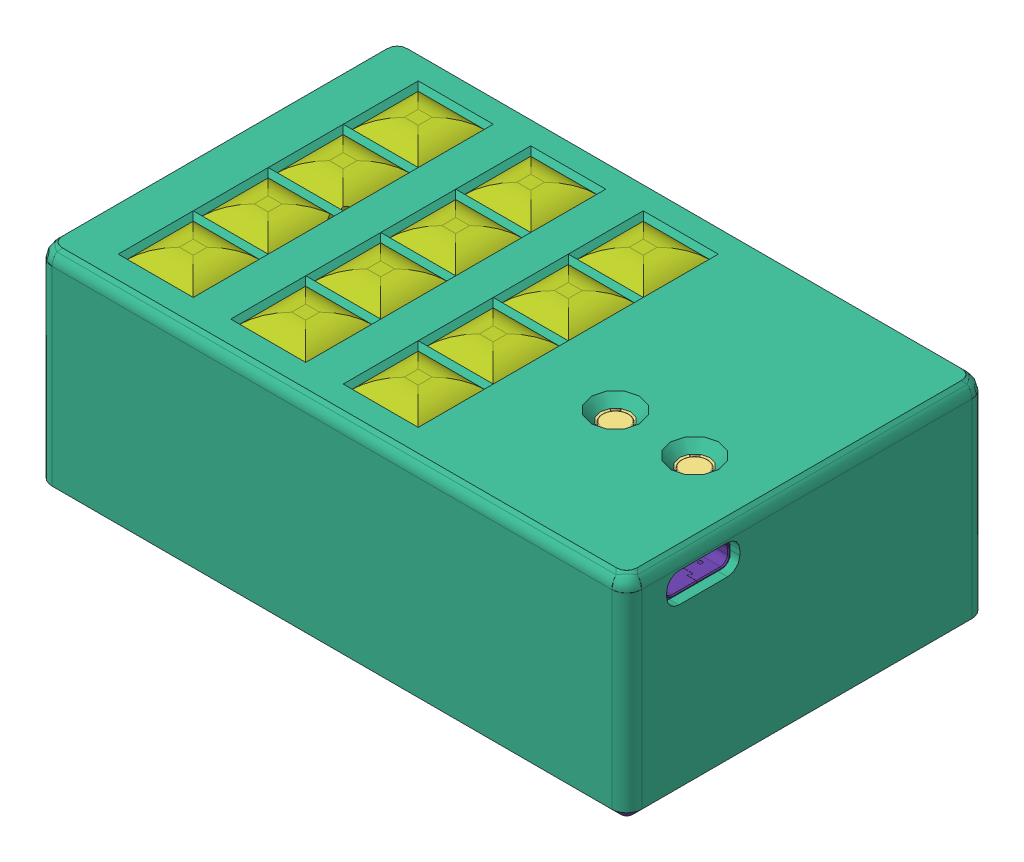
SolidWorks assembly case_mood, configuration Default. Lengths in mm.
Overall size (78.6 29.2 48).
109 component instances, 27 part files, 18 mates.
Components (placement in the parent):
- mood-mood.step-1: mood-mood.step [Default] at (29.4 28.6305 75.6923) x (-1 0 0) z (0 1 0) size (76.01 40 14.44)
  - Board_Geoms_e038.step-1: Board_Geoms_e038.step [Default] at origin size (75 40 1.6)
    - Pcb_e038.step-1: Pcb_e038.step [Default] at (-147.1 99.5 0) size (75 40 1.6)
  - Step_Models_e038.step-1: Step_Models_e038.step [Default] at origin size (71.91 38.55 14.44)
    - Top_e038.step-1: Top_e038.step [Default] at origin size (71.91 38.55 7.8)
      - IC2_DRL0006A_ASM_d850ca76bd89.step-1: IC2_DRL0006A_ASM_d850ca76bd89.step [Default] at (-11.65 2.75 0) size (1.6 1.6 0.6)
        - FRAME-DRL0006A.step-1: FRAME-DRL0006A.step [Default] x (0 1 0) z (1 0 0) size (1.2 0.13 1.6)
          - SOLID.step-1: SOLID.step [Default] at origin size (0.2 0.13 0.3)
          - SOLID001.step-1: SOLID001.step [Default] at origin size (0.2 0.13 0.3)
          - SOLID002.step-1: SOLID002.step [Default] at origin size (0.2 0.13 0.3)
          - SOLID003.step-1: SOLID003.step [Default] at origin size (0.2 0.13 0.3)
          - SOLID004.step-1: SOLID004.step [Default] at origin size (0.2 0.13 0.3)
          - SOLID005.step-1: SOLID005.step [Default] at origin size (0.2 0.13 0.3)
        - BODY-SOT.step-1: BODY-SOT.step [Default] at (0 0 0.025) x (0 1 0) z (1 0 0) size (1.6 0.58 1.2)
      - IC6_ASSEMBLY_ace8437915b6.step-1: IC6_ASSEMBLY_ace8437915b6.step [Default] at (-21.4 7.5 0) size (2.1 2 0.6)
        - Body.step-1: Body.step [Default] at origin size (2 2 0.55)
        - ThermalPin.step-1: ThermalPin.step [Default] at (-0.3875 -0.8375 0) size (0.78 1.68 0.07)
        - PinsArrayLR.step-1: PinsArrayLR.step [Default] at origin size (2.1 1.24 0.07)
      - R52_R_0402_1005Metric_0573c14c30cb.step-1: R52_R_0402_1005Metric_0573c14c30cb.step [Default] at (15.2 -25 0) x (-1 0 0) z (0 0 1) size (1 0.5 0.35)
      - R52_R_0402_1005Metric_0573c14c30cb.step-2: R52_R_0402_1005Metric_0573c14c30cb.step [Default] at (30.2 6.8 0) x (-1 0 0) z (0 0 1) size (1 0.5 0.35)
      - R52_R_0402_1005Metric_0573c14c30cb.step-3: R52_R_0402_1005Metric_0573c14c30cb.step [Default] at (15.2 -6.8 0) x (-1 0 0) z (0 0 1) size (1 0.5 0.35)
      - D4_LED_RGB_5050_6_5aed774da48c.step-1: D4_LED_RGB_5050_6_5aed774da48c.step [Default] at (25 5 0) size (5.4 5 1.6)
      - R52_R_0402_1005Metric_0573c14c30cb.step-4: R52_R_0402_1005Metric_0573c14c30cb.step [Default] at (0.2 -23.2 0) x (-1 0 0) z (0 0 1) size (1 0.5 0.35)
      - IC1_ESP32-C3-WROOM-02-H4_28caeafe01dd.step-1: IC1_ESP32-C3-WROOM-02-H4_28caeafe01dd.step [Default] at (-26.65 -20 0.4) x (-1 0 0) z (0 0 1) size (18 20 3.2)
      - R2_R_0603_1608Metric_003f984474a4.step-1: R2_R_0603_1608Metric_003f984474a4.step [Default] at (-8.65 0 0) x (0 -1 0) z (0 0 1) size (1.6 0.8 0.45)
      - C5_C_0805_2012Metric_cb7698a6af10.step-1: C5_C_0805_2012Metric_cb7698a6af10.step [Default] at (-11.65 0.25 0) size (2 1.25 1.25)
      - R52_R_0402_1005Metric_0573c14c30cb.step-5: R52_R_0402_1005Metric_0573c14c30cb.step [Default] at (30.4 -13.2 0) x (-1 0 0) z (0 0 1) size (1 0.5 0.35)
      - D4_LED_RGB_5050_6_5aed774da48c.step-2: D4_LED_RGB_5050_6_5aed774da48c.step [Default] at (-5 5 0) size (5.4 5 1.6)
      - R52_R_0402_1005Metric_0573c14c30cb.step-6: R52_R_0402_1005Metric_0573c14c30cb.step [Default] at (15.2 -5 0) x (-1 0 0) z (0 0 1) size (1 0.5 0.35)
      - D4_LED_RGB_5050_6_5aed774da48c.step-3: D4_LED_RGB_5050_6_5aed774da48c.step [Default] at (-5 -15 0) size (5.4 5 1.6)
      - R52_R_0402_1005Metric_0573c14c30cb.step-7: R52_R_0402_1005Metric_0573c14c30cb.step [Default] at (15.2 3.2 0) x (-1 0 0) z (0 0 1) size (1 0.5 0.35)
      - D4_LED_RGB_5050_6_5aed774da48c.step-4: D4_LED_RGB_5050_6_5aed774da48c.step [Default] at (10 -15 0) size (5.4 5 1.6)
      - R2_R_0603_1608Metric_003f984474a4.step-2: R2_R_0603_1608Metric_003f984474a4.step [Default] at (-38.1 -17.8 0) x (0 1 0) z (0 0 1) size (1.6 0.8 0.45)
      - R52_R_0402_1005Metric_0573c14c30cb.step-8: R52_R_0402_1005Metric_0573c14c30cb.step [Default] at (30.4 -3.2 0) x (-1 0 0) z (0 0 1) size (1 0.5 0.35)
      - J2_12401610E42A_931c68c1d1c5[2].step-1: J2_12401610E42A_931c68c1d1c5[2].step [Default] at (-41 3.8 1.5) x (-1 0 0) z (0 0 1) size (10.51 9.21 4.22)
      - R2_R_0603_1608Metric_003f984474a4.step-3: R2_R_0603_1608Metric_003f984474a4.step [Default] at (-19 1.6 0) x (0 -1 0) z (0 0 1) size (1.6 0.8 0.45)
      - D4_LED_RGB_5050_6_5aed774da48c.step-5: D4_LED_RGB_5050_6_5aed774da48c.step [Default] at (10 -25 0) size (5.4 5 1.6)
      - R52_R_0402_1005Metric_0573c14c30cb.step-9: R52_R_0402_1005Metric_0573c14c30cb.step [Default] at (30.4 -16.8 0) x (-1 0 0) z (0 0 1) size (1 0.5 0.35)
      - R2_R_0603_1608Metric_003f984474a4.step-4: R2_R_0603_1608Metric_003f984474a4.step [Default] at (-4.65 0.75 0) x (-1 0 0) z (0 0 1) size (1.6 0.8 0.45)
      - R52_R_0402_1005Metric_0573c14c30cb.step-10: R52_R_0402_1005Metric_0573c14c30cb.step [Default] at (15.2025 5 0) x (-1 0 0) z (0 0 1) size (1 0.5 0.35)
      - R2_R_0603_1608Metric_003f984474a4.step-5: R2_R_0603_1608Metric_003f984474a4.step [Default] at (4.5875 -7.2687 0) size (1.6 0.8 0.45)
      - D2_LED_0805_2012Metric_59915ddbd9d1.step-1: D2_LED_0805_2012Metric_59915ddbd9d1.step [Default] at (-21 1.6 0) x (0 -1 0) z (0 0 1) size (2 1.25 1.1)
      - D4_LED_RGB_5050_6_5aed774da48c.step-6: D4_LED_RGB_5050_6_5aed774da48c.step [Default] at (-5 -25 0) size (5.4 5 1.6)
      - R52_R_0402_1005Metric_0573c14c30cb.step-11: R52_R_0402_1005Metric_0573c14c30cb.step [Default] at (0.2 -25 0) x (-1 0 0) z (0 0 1) size (1 0.5 0.35)
      - R52_R_0402_1005Metric_0573c14c30cb.step-12: R52_R_0402_1005Metric_0573c14c30cb.step [Default] at (0.2 3.2 0) x (-1 0 0) z (0 0 1) size (1 0.5 0.35)
      - R52_R_0402_1005Metric_0573c14c30cb.step-13: R52_R_0402_1005Metric_0573c14c30cb.step [Default] at (15.2 -23.2 0) x (-1 0 0) z (0 0 1) size (1 0.5 0.35)
      - R2_R_0603_1608Metric_003f984474a4.step-6: R2_R_0603_1608Metric_003f984474a4.step [Default] at (-14.3 -20.8 0) x (-1 0 0) z (0 0 1) size (1.6 0.8 0.45)
      - R52_R_0402_1005Metric_0573c14c30cb.step-14: R52_R_0402_1005Metric_0573c14c30cb.step [Default] at (30.4 -25 0) x (-1 0 0) z (0 0 1) size (1 0.5 0.35)
      - C11_C_0603_1608Metric_8816bd15a2e3.step-1: C11_C_0603_1608Metric_8816bd15a2e3.step [Default] at (-18.65 7.75 0) x (0 1 0) z (0 0 1) size (1.6 0.8 0.8)
      - D4_LED_RGB_5050_6_5aed774da48c.step-7: D4_LED_RGB_5050_6_5aed774da48c.step [Default] at (25 -25 0) size (5.4 5 1.6)
      - R52_R_0402_1005Metric_0573c14c30cb.step-15: R52_R_0402_1005Metric_0573c14c30cb.step [Default] at (0.2 -3.2 0) x (-1 0 0) z (0 0 1) size (1 0.5 0.35)
      - R2_R_0603_1608Metric_003f984474a4.step-7: R2_R_0603_1608Metric_003f984474a4.step [Default] at (-27.2 0.8 0) x (0 1 0) z (0 0 1) size (1.6 0.8 0.45)
      - C11_C_0603_1608Metric_8816bd15a2e3.step-2: C11_C_0603_1608Metric_8816bd15a2e3.step [Default] at (-11.65 -4 0) size (1.6 0.8 0.8)
      - R52_R_0402_1005Metric_0573c14c30cb.step-16: R52_R_0402_1005Metric_0573c14c30cb.step [Default] at (30.4 -15 0) x (-1 0 0) z (0 0 1) size (1 0.5 0.35)
      - R52_R_0402_1005Metric_0573c14c30cb.step-17: R52_R_0402_1005Metric_0573c14c30cb.step [Default] at (0.2 5 0) x (-1 0 0) z (0 0 1) size (1 0.5 0.35)
      - C11_C_0603_1608Metric_8816bd15a2e3.step-3: C11_C_0603_1608Metric_8816bd15a2e3.step [Default] at (-7.15 0 0) x (0 1 0) z (0 0 1) size (1.6 0.8 0.8)
      - R52_R_0402_1005Metric_0573c14c30cb.step-18: R52_R_0402_1005Metric_0573c14c30cb.step [Default] at (0.2 -6.8 0) x (-1 0 0) z (0 0 1) size (1 0.5 0.35)
      - R2_R_0603_1608Metric_003f984474a4.step-8: R2_R_0603_1608Metric_003f984474a4.step [Default] at (-14.3 -14.4 0) x (-1 0 0) z (0 0 1) size (1.6 0.8 0.45)
      - D4_LED_RGB_5050_6_5aed774da48c.step-8: D4_LED_RGB_5050_6_5aed774da48c.step [Default] at (25 -15 0) size (5.4 5 1.6)
      - R52_R_0402_1005Metric_0573c14c30cb.step-19: R52_R_0402_1005Metric_0573c14c30cb.step [Default] at (30.2 5 0) x (-1 0 0) z (0 0 1) size (1 0.5 0.35)
      - R2_R_0603_1608Metric_003f984474a4.step-9: R2_R_0603_1608Metric_003f984474a4.step [Default] at (4.5875 -17.2063 0) size (1.6 0.8 0.45)
      - D4_LED_RGB_5050_6_5aed774da48c.step-9: D4_LED_RGB_5050_6_5aed774da48c.step [Default] at (10 -5 0) size (5.4 5 1.6)
      - R2_R_0603_1608Metric_003f984474a4.step-10: R2_R_0603_1608Metric_003f984474a4.step [Default] at (-14.3 -17.6 0) size (1.6 0.8 0.45)
      - R2_R_0603_1608Metric_003f984474a4.step-11: R2_R_0603_1608Metric_003f984474a4.step [Default] at (-25.2 1.6 0) x (0 -1 0) z (0 0 1) size (1.6 0.8 0.45)
      - R52_R_0402_1005Metric_0573c14c30cb.step-20: R52_R_0402_1005Metric_0573c14c30cb.step [Default] at (30.4 -6.8 0) x (-1 0 0) z (0 0 1) size (1 0.5 0.35)
      - R2_R_0603_1608Metric_003f984474a4.step-12: R2_R_0603_1608Metric_003f984474a4.step [Default] at (-38.1 -14.4 0) x (0 1 0) z (0 0 1) size (1.6 0.8 0.45)
      - R52_R_0402_1005Metric_0573c14c30cb.step-21: R52_R_0402_1005Metric_0573c14c30cb.step [Default] at (15.2 6.8 0) x (-1 0 0) z (0 0 1) size (1 0.5 0.35)
      - R52_R_0402_1005Metric_0573c14c30cb.step-22: R52_R_0402_1005Metric_0573c14c30cb.step [Default] at (15.2025 -3.2 0) x (-1 0 0) z (0 0 1) size (1 0.5 0.35)
      - R52_R_0402_1005Metric_0573c14c30cb.step-23: R52_R_0402_1005Metric_0573c14c30cb.step [Default] at (30.2 3.2 0) x (-1 0 0) z (0 0 1) size (1 0.5 0.35)
      - Q2_SOT_23_dd72da5cd8d7.step-1: Q2_SOT_23_dd72da5cd8d7.step [Default] at (4.55 -24.1188 0) x (0 1 0) z (0 0 1) size (2.5 3 1.2)
      - R52_R_0402_1005Metric_0573c14c30cb.step-24: R52_R_0402_1005Metric_0573c14c30cb.step [Default] at (30.4 -26.8 0) x (-1 0 0) z (0 0 1) size (1 0.5 0.35)
      - C11_C_0603_1608Metric_8816bd15a2e3.step-4: C11_C_0603_1608Metric_8816bd15a2e3.step [Default] at (-11.7 -19.9 0) x (0 1 0) z (0 0 1) size (1.6 0.8 0.8)
      - R2_R_0603_1608Metric_003f984474a4.step-13: R2_R_0603_1608Metric_003f984474a4.step [Default] at (-38.1 -21.3 0) x (0 1 0) z (0 0 1) size (1.6 0.8 0.45)
      - C5_C_0805_2012Metric_cb7698a6af10.step-2: C5_C_0805_2012Metric_cb7698a6af10.step [Default] at (-10.65 7 0) size (2 1.25 1.25)
      - SW2_SW_PUSH_6mm_h4.3mm_68b5b15dd36c.step-1: SW2_SW_PUSH_6mm_h4.3mm_68b5b15dd36c.step [Default] at (-18 -7.4 0) x (-1 0 0) z (0 0 1) size (7.17 6 7.8)
      - R52_R_0402_1005Metric_0573c14c30cb.step-25: R52_R_0402_1005Metric_0573c14c30cb.step [Default] at (15.2 -13.2 0) x (-1 0 0) z (0 0 1) size (1 0.5 0.35)
      - R52_R_0402_1005Metric_0573c14c30cb.step-26: R52_R_0402_1005Metric_0573c14c30cb.step [Default] at (15.2 -26.8 0) x (-1 0 0) z (0 0 1) size (1 0.5 0.35)
      - R2_R_0603_1608Metric_003f984474a4.step-14: R2_R_0603_1608Metric_003f984474a4.step [Default] at (-21.4 5.25 0) size (1.6 0.8 0.45)
      - C11_C_0603_1608Metric_8816bd15a2e3.step-5: C11_C_0603_1608Metric_8816bd15a2e3.step [Default] at (-14.3 -22.5 0) size (1.6 0.8 0.8)
      - D4_LED_RGB_5050_6_5aed774da48c.step-10: D4_LED_RGB_5050_6_5aed774da48c.step [Default] at (25 -5 0) size (5.4 5 1.6)
      - SW2_SW_PUSH_6mm_h4.3mm_68b5b15dd36c.step-2: SW2_SW_PUSH_6mm_h4.3mm_68b5b15dd36c.step [Default] at (-34.85 -2.9 0) size (7.17 6 7.8)
      - R52_R_0402_1005Metric_0573c14c30cb.step-27: R52_R_0402_1005Metric_0573c14c30cb.step [Default] at (0.2 -5 0) x (-1 0 0) z (0 0 1) size (1 0.5 0.35)
      - R2_R_0603_1608Metric_003f984474a4.step-15: R2_R_0603_1608Metric_003f984474a4.step [Default] at (-29 0.8 0) x (0 1 0) z (0 0 1) size (1.6 0.8 0.45)
      - C5_C_0805_2012Metric_cb7698a6af10.step-3: C5_C_0805_2012Metric_cb7698a6af10.step [Default] at (-11.65 -2 0) size (2 1.25 1.25)
      - D4_LED_RGB_5050_6_5aed774da48c.step-11: D4_LED_RGB_5050_6_5aed774da48c.step [Default] at (10 5 0) size (5.4 5 1.6)
      - R52_R_0402_1005Metric_0573c14c30cb.step-28: R52_R_0402_1005Metric_0573c14c30cb.step [Default] at (15.2 -16.8 0) x (-1 0 0) z (0 0 1) size (1 0.5 0.35)
      - L1_L_Wuerth_MAPI_4020_5ef69c3bf382.step-1: L1_L_Wuerth_MAPI_4020_5ef69c3bf382.step [Default] at (-15.65 1.75 0) x (0 1 0) z (0 0 1) size (3 4 2)
      - R2_R_0603_1608Metric_003f984474a4.step-16: R2_R_0603_1608Metric_003f984474a4.step [Default] at (-14.3 -19.2 0) x (-1 0 0) z (0 0 1) size (1.6 0.8 0.45)
      - R52_R_0402_1005Metric_0573c14c30cb.step-29: R52_R_0402_1005Metric_0573c14c30cb.step [Default] at (30.4 -23.2 0) x (-1 0 0) z (0 0 1) size (1 0.5 0.35)
      - Q2_SOT_23_dd72da5cd8d7.step-2: Q2_SOT_23_dd72da5cd8d7.step [Default] at (4.55 -4.0688 0) x (0 1 0) z (0 0 1) size (2.5 3 1.2)
      - D4_LED_RGB_5050_6_5aed774da48c.step-12: D4_LED_RGB_5050_6_5aed774da48c.step [Default] at (-5 -5 0) size (5.4 5 1.6)
      - C11_C_0603_1608Metric_8816bd15a2e3.step-6: C11_C_0603_1608Metric_8816bd15a2e3.step [Default] at (-10.65 5 0) size (1.6 0.8 0.8)
      - R52_R_0402_1005Metric_0573c14c30cb.step-30: R52_R_0402_1005Metric_0573c14c30cb.step [Default] at (0.2 -13.2 0) x (-1 0 0) z (0 0 1) size (1 0.5 0.35)
      - R52_R_0402_1005Metric_0573c14c30cb.step-31: R52_R_0402_1005Metric_0573c14c30cb.step [Default] at (0.2 -15 0) x (-1 0 0) z (0 0 1) size (1 0.5 0.35)
      - R52_R_0402_1005Metric_0573c14c30cb.step-32: R52_R_0402_1005Metric_0573c14c30cb.step [Default] at (0.2 -26.8 0) x (-1 0 0) z (0 0 1) size (1 0.5 0.35)
      - D2_LED_0805_2012Metric_59915ddbd9d1.step-2: D2_LED_0805_2012Metric_59915ddbd9d1.step [Default] at (-23.2 1.6 0) x (0 -1 0) z (0 0 1) size (2 1.25 1.1)
      - R52_R_0402_1005Metric_0573c14c30cb.step-33: R52_R_0402_1005Metric_0573c14c30cb.step [Default] at (0.2 6.8 0) x (-1 0 0) z (0 0 1) size (1 0.5 0.35)
      - R2_R_0603_1608Metric_003f984474a4.step-17: R2_R_0603_1608Metric_003f984474a4.step [Default] at (4.55 -27.0188 0) size (1.6 0.8 0.45)
      - R52_R_0402_1005Metric_0573c14c30cb.step-34: R52_R_0402_1005Metric_0573c14c30cb.step [Default] at (0.2 -16.8 0) x (-1 0 0) z (0 0 1) size (1 0.5 0.35)
      - Q2_SOT_23_dd72da5cd8d7.step-3: Q2_SOT_23_dd72da5cd8d7.step [Default] at (4.55 -14.0687 0) x (0 1 0) z (0 0 1) size (2.5 3 1.2)
      - R52_R_0402_1005Metric_0573c14c30cb.step-35: R52_R_0402_1005Metric_0573c14c30cb.step [Default] at (15.2 -15 0) x (-1 0 0) z (0 0 1) size (1 0.5 0.35)
      - R52_R_0402_1005Metric_0573c14c30cb.step-36: R52_R_0402_1005Metric_0573c14c30cb.step [Default] at (30.4 -5 0) x (-1 0 0) z (0 0 1) size (1 0.5 0.35)
    - Bot_e038.step-1: Bot_e038.step [Default] at origin size (5.08 7.62 11.54) (hidden)
      - J1_PinHeader_2x03_P254mm_Vertical_e1aae7fb38ca.step-1: J1_PinHeader_2x03_P254mm_Vertical_e1aae7fb38ca.step [Default] at (-24.275 -19.525 -1.6) x (1 0 0) z (0 0 -1) size (5.08 7.62 11.54)
- 18650 v4.step-1: 18650 v4.step [Default] at (-0.7032 16.0125 53.1923) x (0 0 -1) z (1 0 0) size (18 18 65.13)
- 18650 v4.step-2: 18650 v4.step [Default] at (-0.7032 16.0125 78.1923) x (0 0 -1) z (1 0 0) size (18 18 65.13)
- Part25^case_mood-1: Part25^case_mood [Default] at (176.5 27.0305 175.1923) x (1 0 0) z (0 -1 0) size (78.6 48 27.2) (virtual)
- Part26^case_mood-1: Part26^case_mood [Default] at (176.5 33.0305 175.1923) x (1 0 0) z (0 -1 0) size (40 40 4.9) (virtual)
- Part27^case_mood-1: Part27^case_mood [Default] at (176.5 7.0305 175.1923) x (1 0 0) z (0 -1 0) size (78.6 48 8.2) (virtual)
Mates (geometry in assembly coordinates):
- Coincident1: coincident aligned: plane of 18650 v4.step-1 through (-0.7032 16.0125 53.1923) normal (0 1 0); plane of 18650 v4.step-2 through (-0.7032 16.0125 78.1923) normal (0 1 0)
- Distance1: distance = 25 mm aligned: plane of 18650 v4.step-2 through (-0.7032 16.0125 78.1923) normal (0 0 -1); plane of 18650 v4.step-1 through (-0.7032 16.0125 53.1923) normal (0 0 -1)
- Coincident3: coincident aligned: plane of 18650 v4.step-1 through (-0.6032 16.0125 53.1923) normal (-1 0 0); plane of 18650 v4.step-2 through (-0.6032 16.0125 78.1923) normal (-1 0 0)
- Symmetric1: symmetric anti-aligned: plane of 18650 v4.step-1 through (-0.7032 16.0125 53.1923) normal (0 0 -1); plane of 18650 v4.step-2 through (-0.7032 16.0125 78.1923) normal (0 0 -1)
- Symmetric2: symmetric aligned: plane of 18650 v4.step-1 through (-0.6032 16.0125 53.1923) normal (-1 0 0); plane of 18650 v4.step-2 through (64.4031 16.0125 78.1923) normal (1 0 0)
- InPlace1: in place: plane of mood-mood.step-1/Board_Geoms_e038.step-1/Pcb_e038.step-1 through (31.0515 27.0305 66.575) normal (0 -1 0); plane of ? through (0 27.0305 0) normal (0 -1 0); moOrthogonalPlaneRef_w of mood-mood.step-1/Board_Geoms_e038.step-1/Pcb_e038.step-1 through (31.0515 27.0305 66.575) normal (0 -1 0); plane of ? through (0 27.0305 0) normal (0 0 -1); plane of mood-mood.step-1/Board_Geoms_e038.step-1/Pcb_e038.step-1 through (31.0515 27.0305 66.575) normal (0 -1 0); plane of ? through (0 27.0305 0) normal (-1 0 0); plane of mood-mood.step-1/Board_Geoms_e038.step-1/Pcb_e038.step-1 through (31.0515 27.0305 66.575) normal (0 -1 0); unknown of Part25^case_mood-1
- Coincident6: coincident aligned: plane of mood-mood.step-1/Board_Geoms_e038.step-1/Pcb_e038.step-1; plane of Part25^case_mood-1
- Coincident7: coincident aligned: moOrthogonalPlaneRef_w of mood-mood.step-1/Board_Geoms_e038.step-1/Pcb_e038.step-1 through (176.5 27.0305 175.1923) normal (0 0 1); plane of Part25^case_mood-1 through (176.5 27.0305 175.1923) normal (0 0 1)
- Coincident8: coincident anti-aligned: moOrthogonalPlaneRef_w of mood-mood.step-1/Board_Geoms_e038.step-1/Pcb_e038.step-1 through (176.5 27.0305 175.1923) normal (-1 0 0); plane of Part25^case_mood-1 through (176.5 27.0305 175.1923) normal (1 0 0)
- Coincident9: coincident: cylinder of 18650 v4.step-1 through (30.0468 16.0125 53.1923) axis (1 0 0) radius 9; line of Part25^case_mood-1 through (1.3149 25.0125 53.1923) axis (1 0 0)
- InPlace2: in place: plane of Part25^case_mood-1 through (176.5 33.0305 175.1923) normal (0 -1 0); plane of ? through (0 33.0305 0) normal (0 -1 0); plane of Part25^case_mood-1 through (176.5 33.0305 175.1923) normal (0 -1 0); plane of ? through (0 33.0305 0) normal (0 0 -1); plane of Part25^case_mood-1 through (176.5 33.0305 175.1923) normal (0 -1 0); plane of ? through (0 33.0305 0) normal (-1 0 0); plane of Part25^case_mood-1 through (176.5 33.0305 175.1923) normal (0 -1 0); unknown of Part26^case_mood-1
- Coincident10: coincident aligned: plane of Part25^case_mood-1; plane of Part26^case_mood-1
- Coincident11: coincident aligned: moOrthogonalPlaneRef_w of Part25^case_mood-1 through (176.5 33.0305 175.1923) normal (0 0 1); plane of Part26^case_mood-1 through (176.5 33.0305 175.1923) normal (0 0 1)
- Coincident12: coincident anti-aligned: moOrthogonalPlaneRef_w of Part25^case_mood-1 through (176.5 33.0305 175.1923) normal (-1 0 0); plane of Part26^case_mood-1 through (176.5 33.0305 175.1923) normal (1 0 0)
- InPlace3: in place: plane of Part25^case_mood-1 through (176.5 7.0305 175.1923) normal (0 -1 0); plane of ? through (0 7.0305 0) normal (0 -1 0); plane of Part25^case_mood-1 through (176.5 7.0305 175.1923) normal (0 -1 0); plane of ? through (0 7.0305 0) normal (0 0 -1); plane of Part25^case_mood-1 through (176.5 7.0305 175.1923) normal (0 -1 0); plane of ? through (0 7.0305 0) normal (-1 0 0); plane of Part25^case_mood-1 through (176.5 7.0305 175.1923) normal (0 -1 0); unknown of Part27^case_mood-1
- Coincident13: coincident aligned: plane of Part25^case_mood-1; plane of Part27^case_mood-1
- Coincident14: coincident aligned: moOrthogonalPlaneRef_w of Part25^case_mood-1 through (176.5 7.0305 175.1923) normal (0 0 1); plane of Part27^case_mood-1 through (176.5 7.0305 175.1923) normal (0 0 1)
- Coincident15: coincident anti-aligned: moOrthogonalPlaneRef_w of Part25^case_mood-1 through (176.5 7.0305 175.1923) normal (-1 0 0); plane of Part27^case_mood-1 through (176.5 7.0305 175.1923) normal (1 0 0)
